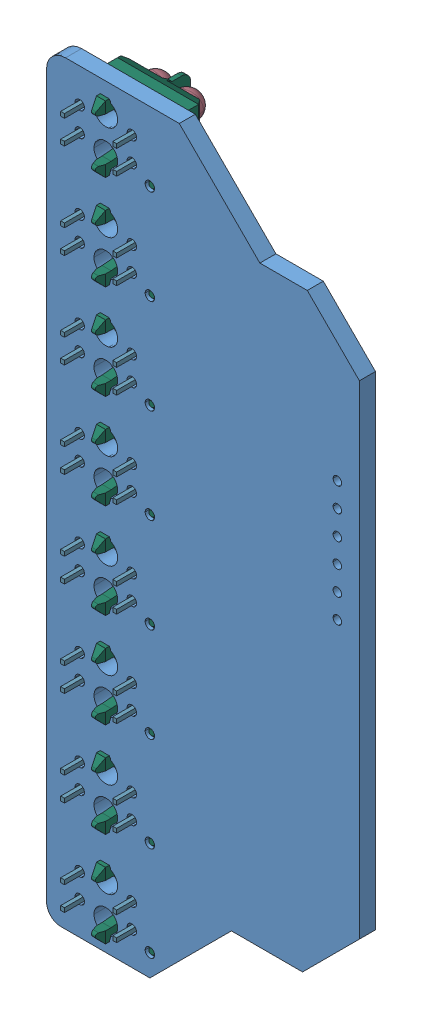
SolidWorks assembly Linelance_PCB v1.1, configuration По умолчанию. Lengths in mm.
Overall size (33 79.6 10.52).
455 component instances, 37 part files, 0 mates.
Components (placement in the parent):
- Linelance_PCB v1.1.step-1: Linelance_PCB v1.1.step [По умолчанию] at origin size (33 79.6 10.52)
  - Linelance_PCB v1.1.step.step-1: Linelance_PCB v1.1.step.step [По умолчанию] at origin size (33 79.6 10.52)
    - Board.step.step-1: Board.step.step [По умолчанию] at origin size (33 79.6 1.69)
      - Open CASCADE STEP translator 6.8 2.1.1.step.step-1: Open CASCADE STEP translator 6.8 2.1.1.step.step [По умолчанию] at (0 0 -1.692) size (33 79.6 1.69)
    - C16.step.step-1: C16.step.step [По умолчанию] at origin size (1.6 0.8 0.5)
      - 5899458880.step.step-1: 5899458880.step.step [По умолчанию] at (18.6 33.5 -2.192) size (1 0.8 0.5)
        - Extruded.step.step-1: Extruded.step.step [По умолчанию] at origin size (1 0.8 0.5)
      - 5899458400.step.step-1: 5899458400.step.step [По умолчанию] at (19.25 33.5 -2.192) size (0.3 0.8 0.5)
        - Extruded-0.step.step-1: Extruded-0.step.step [По умолчанию] at origin size (0.3 0.8 0.5)
      - 5899458400.step-1.step-1: 5899458400.step-1.step [По умолчанию] at (17.95 33.5 -2.192) size (0.3 0.8 0.5)
        - Extruded-0.step.step-1: Extruded-0.step.step [По умолчанию] at origin size (0.3 0.8 0.5)
    - C15.step.step-1: C15.step.step [По умолчанию] at origin size (1.6 0.8 0.5)
      - 5899458880.step-1.step-1: 5899458880.step-1.step [По умолчанию] at (18.6 34.8 -2.192) size (1 0.8 0.5)
        - Extruded.step.step-1: Extruded.step.step [По умолчанию] at origin size (1 0.8 0.5)
      - 5899458400.step-2.step-1: 5899458400.step-2.step [По умолчанию] at (19.25 34.8 -2.192) size (0.3 0.8 0.5)
        - Extruded-0.step.step-1: Extruded-0.step.step [По умолчанию] at origin size (0.3 0.8 0.5)
      - 5899458400.step-3.step-1: 5899458400.step-3.step [По умолчанию] at (17.95 34.8 -2.192) size (0.3 0.8 0.5)
        - Extruded-0.step.step-1: Extruded-0.step.step [По умолчанию] at origin size (0.3 0.8 0.5)
    - C11.step.step-1: C11.step.step [По умолчанию] at origin size (0.8 1.6 0.5)
      - 5899457520.step.step-1: 5899457520.step.step [По умолчанию] at (26.2 43.7 -2.192) size (0.8 1 0.5)
        - Extruded-1.step.step-1: Extruded-1.step.step [По умолчанию] at origin size (0.8 1 0.5)
      - 5899457200.step.step-1: 5899457200.step.step [По умолчанию] at (26.2 43.05 -2.192) size (0.8 0.3 0.5)
        - Extruded-2.step.step-1: Extruded-2.step.step [По умолчанию] at origin size (0.8 0.3 0.5)
      - 5899457200.step-1.step-1: 5899457200.step-1.step [По умолчанию] at (26.2 44.35 -2.192) size (0.8 0.3 0.5)
        - Extruded-2.step.step-1: Extruded-2.step.step [По умолчанию] at origin size (0.8 0.3 0.5)
    - R1.step.step-1: R1.step.step [По умолчанию] at origin size (1.6 0.8 0.5)
      - 5770196880.step.step-1: 5770196880.step.step [По умолчанию] at (26.3 33.7 -1.692) x (-1 0 0) z (0 0 -1) size (1.6 0.8 0.5)
        - Terminal.step.step-1: Terminal.step.step [По умолчанию] at (-0.8 -0.4 0) size (0.3 0.8 0.5)
          - Open_CASCADE_STEP_translator_6.8_7.2.1.step.step-1: Open_CASCADE_STEP_translator_6.8_7.2.1.step.step [По умолчанию] at origin size (0.3 0.8 0.5)
        - Terminal.step-1.step-1: Terminal.step-1.step [По умолчанию] at (0.8 0.4 0) x (-1 0 0) z (0 0 1) size (0.3 0.8 0.5)
          - Open_CASCADE_STEP_translator_6.8_7.2.1.step.step-1: Open_CASCADE_STEP_translator_6.8_7.2.1.step.step [По умолчанию] at origin size (0.3 0.8 0.5)
        - Mid_Body.step.step-1: Mid_Body.step.step [По умолчанию] at (-0.8 -0.4 0) size (1.5 0.8 0.4)
        - Mark.step.step-1: Mark.step.step [По умолчанию] at (-0.5 -0.4 0.45) size (1 0.8 0.05)
    - Y1.step.step-1: Y1.step.step [По умолчанию] at origin size (3.2 2.5 0.6)
      - TSX-3225.step.step-1: TSX-3225.step.step [По умолчанию] at (23.15 31 -1.692) x (1 0 0) z (0 0 -1) size (3.2 2.5 0.6)
    - RN2.step.step-1: RN2.step.step [По умолчанию] at origin size (1.85 3.35 0.7)
      - 5770195440.step.step-1: 5770195440.step.step [По умолчанию] at (13.2 19.25 -1.692) x (1 0 0) z (0 0 -1) size (1.85 3.35 0.7)
        - body.step.step-1: body.step.step [По умолчанию] at (-0.875 -1.675 0) size (1.75 3.35 0.6)
          - Open_CASCADE_STEP_translator_6.8_25.1.1.step.step-1: Open_CASCADE_STEP_translator_6.8_25.1.1.step.step [По умолчанию] at origin size (1.75 3.35 0.6)
        - Mid_Pin.step.step-1: Mid_Pin.step.step [По умолчанию] at (-0.875 -1.2 0) size (0.3 0.38 0.7)
          - Open_CASCADE_STEP_translator_6.8_25.3.1.step.step-1: Open_CASCADE_STEP_translator_6.8_25.3.1.step.step [По умолчанию] at origin size (0.3 0.38 0.7)
        - Mid_Pin.step-1.step-1: Mid_Pin.step-1.step [По умолчанию] at (0.875 1.2 0) x (-1 0 0) z (0 0 1) size (0.3 0.38 0.7)
          - Open_CASCADE_STEP_translator_6.8_25.3.1.step.step-1: Open_CASCADE_STEP_translator_6.8_25.3.1.step.step [По умолчанию] at origin size (0.3 0.38 0.7)
        - Mid_Pin.step-2.step-1: Mid_Pin.step-2.step [По умолчанию] at (-0.875 -0.4 0) size (0.3 0.38 0.7)
          - Open_CASCADE_STEP_translator_6.8_25.3.1.step.step-1: Open_CASCADE_STEP_translator_6.8_25.3.1.step.step [По умолчанию] at origin size (0.3 0.38 0.7)
        - Mid_Pin.step-3.step-1: Mid_Pin.step-3.step [По умолчанию] at (0.875 0.4 0) x (-1 0 0) z (0 0 1) size (0.3 0.38 0.7)
          - Open_CASCADE_STEP_translator_6.8_25.3.1.step.step-1: Open_CASCADE_STEP_translator_6.8_25.3.1.step.step [По умолчанию] at origin size (0.3 0.38 0.7)
        - Mid_Pin.step-4.step-1: Mid_Pin.step-4.step [По умолчанию] at (-0.875 0.4 0) size (0.3 0.38 0.7)
          - Open_CASCADE_STEP_translator_6.8_25.3.1.step.step-1: Open_CASCADE_STEP_translator_6.8_25.3.1.step.step [По умолчанию] at origin size (0.3 0.38 0.7)
        - Mid_Pin.step-5.step-1: Mid_Pin.step-5.step [По умолчанию] at (0.875 -0.4 0) x (-1 0 0) z (0 0 1) size (0.3 0.38 0.7)
          - Open_CASCADE_STEP_translator_6.8_25.3.1.step.step-1: Open_CASCADE_STEP_translator_6.8_25.3.1.step.step [По умолчанию] at origin size (0.3 0.38 0.7)
        - Mid_Pin.step-6.step-1: Mid_Pin.step-6.step [По умолчанию] at (-0.875 1.2 0) size (0.3 0.38 0.7)
          - Open_CASCADE_STEP_translator_6.8_25.3.1.step.step-1: Open_CASCADE_STEP_translator_6.8_25.3.1.step.step [По умолчанию] at origin size (0.3 0.38 0.7)
        - Mid_Pin.step-7.step-1: Mid_Pin.step-7.step [По умолчанию] at (0.875 -1.2 0) x (-1 0 0) z (0 0 1) size (0.3 0.38 0.7)
          - Open_CASCADE_STEP_translator_6.8_25.3.1.step.step-1: Open_CASCADE_STEP_translator_6.8_25.3.1.step.step [По умолчанию] at origin size (0.3 0.38 0.7)
        - Mark.step.step-1: Mark.step.step [По умолчанию] at (-0.875 -1.675 0) size (1 0.8 0.05)
    - RN1.step.step-1: RN1.step.step [По умолчанию] at origin size (1.85 3.35 0.7)
      - 5770195440.step-1.step-1: 5770195440.step-1.step [По умолчанию] at (13.3 61.4 -1.692) x (1 0 0) z (0 0 -1) size (1.85 3.35 0.7)
        - body.step-1.step-1: body.step-1.step [По умолчанию] at (-0.875 -1.675 0) size (1.75 3.35 0.6)
          - Open_CASCADE_STEP_translator_6.8_25.1.1.step.step-1: Open_CASCADE_STEP_translator_6.8_25.1.1.step.step [По умолчанию] at origin size (1.75 3.35 0.6)
        - Mid_Pin.step-8.step-1: Mid_Pin.step-8.step [По умолчанию] at (-0.875 -1.2 0) size (0.3 0.38 0.7)
          - Open_CASCADE_STEP_translator_6.8_25.3.1.step.step-1: Open_CASCADE_STEP_translator_6.8_25.3.1.step.step [По умолчанию] at origin size (0.3 0.38 0.7)
        - Mid_Pin.step-9.step-1: Mid_Pin.step-9.step [По умолчанию] at (0.875 1.2 0) x (-1 0 0) z (0 0 1) size (0.3 0.38 0.7)
          - Open_CASCADE_STEP_translator_6.8_25.3.1.step.step-1: Open_CASCADE_STEP_translator_6.8_25.3.1.step.step [По умолчанию] at origin size (0.3 0.38 0.7)
        - Mid_Pin.step-10.step-1: Mid_Pin.step-10.step [По умолчанию] at (-0.875 -0.4 0) size (0.3 0.38 0.7)
          - Open_CASCADE_STEP_translator_6.8_25.3.1.step.step-1: Open_CASCADE_STEP_translator_6.8_25.3.1.step.step [По умолчанию] at origin size (0.3 0.38 0.7)
        - Mid_Pin.step-11.step-1: Mid_Pin.step-11.step [По умолчанию] at (0.875 0.4 0) x (-1 0 0) z (0 0 1) size (0.3 0.38 0.7)
          - Open_CASCADE_STEP_translator_6.8_25.3.1.step.step-1: Open_CASCADE_STEP_translator_6.8_25.3.1.step.step [По умолчанию] at origin size (0.3 0.38 0.7)
        - Mid_Pin.step-12.step-1: Mid_Pin.step-12.step [По умолчанию] at (-0.875 0.4 0) size (0.3 0.38 0.7)
          - Open_CASCADE_STEP_translator_6.8_25.3.1.step.step-1: Open_CASCADE_STEP_translator_6.8_25.3.1.step.step [По умолчанию] at origin size (0.3 0.38 0.7)
        - Mid_Pin.step-13.step-1: Mid_Pin.step-13.step [По умолчанию] at (0.875 -0.4 0) x (-1 0 0) z (0 0 1) size (0.3 0.38 0.7)
          - Open_CASCADE_STEP_translator_6.8_25.3.1.step.step-1: Open_CASCADE_STEP_translator_6.8_25.3.1.step.step [По умолчанию] at origin size (0.3 0.38 0.7)
        - Mid_Pin.step-14.step-1: Mid_Pin.step-14.step [По умолчанию] at (-0.875 1.2 0) size (0.3 0.38 0.7)
          - Open_CASCADE_STEP_translator_6.8_25.3.1.step.step-1: Open_CASCADE_STEP_translator_6.8_25.3.1.step.step [По умолчанию] at origin size (0.3 0.38 0.7)
        - Mid_Pin.step-15.step-1: Mid_Pin.step-15.step [По умолчанию] at (0.875 -1.2 0) x (-1 0 0) z (0 0 1) size (0.3 0.38 0.7)
          - Open_CASCADE_STEP_translator_6.8_25.3.1.step.step-1: Open_CASCADE_STEP_translator_6.8_25.3.1.step.step [По умолчанию] at origin size (0.3 0.38 0.7)
        - Mark.step.step-1: Mark.step.step [По умолчанию] at (-0.875 -1.675 0) size (1 0.8 0.05)
    - C23.step.step-1: C23.step.step [По умолчанию] at origin size (1.6 0.8 0.5)
      - 5899458400.step-4.step-1: 5899458400.step-4.step [По умолчанию] at (17.5 13.375 -2.192) size (0.3 0.8 0.5)
        - Extruded-0.step.step-1: Extruded-0.step.step [По умолчанию] at origin size (0.3 0.8 0.5)
      - 5899458400.step-5.step-1: 5899458400.step-5.step [По умолчанию] at (16.2 13.375 -2.192) size (0.3 0.8 0.5)
        - Extruded-0.step.step-1: Extruded-0.step.step [По умолчанию] at origin size (0.3 0.8 0.5)
      - 5899458880.step-2.step-1: 5899458880.step-2.step [По умолчанию] at (16.85 13.375 -2.192) size (1 0.8 0.5)
        - Extruded.step.step-1: Extruded.step.step [По умолчанию] at origin size (1 0.8 0.5)
    - C22.step.step-1: C22.step.step [По умолчанию] at origin size (1.6 0.8 0.5)
      - 5899458400.step-6.step-1: 5899458400.step-6.step [По умолчанию] at (17.625 57.7 -2.192) size (0.3 0.8 0.5)
        - Extruded-0.step.step-1: Extruded-0.step.step [По умолчанию] at origin size (0.3 0.8 0.5)
      - 5899458400.step-7.step-1: 5899458400.step-7.step [По умолчанию] at (16.325 57.7 -2.192) size (0.3 0.8 0.5)
        - Extruded-0.step.step-1: Extruded-0.step.step [По умолчанию] at origin size (0.3 0.8 0.5)
      - 5899458880.step-3.step-1: 5899458880.step-3.step [По умолчанию] at (16.975 57.7 -2.192) size (1 0.8 0.5)
        - Extruded.step.step-1: Extruded.step.step [По умолчанию] at origin size (1 0.8 0.5)
    - Q9.step.step-1: Q9.step.step [По умолчанию] at origin size (2.3 2.9 1)
      - SOT23-3.step.step-1: SOT23-3.step.step [По умолчанию] at (13.2 10.85 -1.692) x (0 -1 0) z (1 0 0) size (2.9 1 2.3)
    - Q8.step.step-1: Q8.step.step [По умолчанию] at origin size (2.9 2.3 1)
      - SOT23-3.step.step-1: SOT23-3.step.step [По умолчанию] at (14.75 14.925 -1.692) x (-1 0 0) z (0 -1 0) size (2.9 1 2.3)
    - Q7.step.step-1: Q7.step.step [По умолчанию] at origin size (2.9 2.3 1)
      - SOT23-3.step.step-1: SOT23-3.step.step [По умолчанию] at (15 25.2 -1.692) x (-1 0 0) z (0 -1 0) size (2.9 1 2.3)
    - Q6.step.step-1: Q6.step.step [По умолчанию] at origin size (2.9 2.3 1)
      - SOT23-3.step.step-1: SOT23-3.step.step [По умолчанию] at (15 35.2 -1.692) x (-1 0 0) z (0 -1 0) size (2.9 1 2.3)
    - Q4.step.step-1: Q4.step.step [По умолчанию] at origin size (2.9 2.3 1)
      - SOT23-3.step.step-1: SOT23-3.step.step [По умолчанию] at (15.05 55 -1.692) x (-1 0 0) z (0 -1 0) size (2.9 1 2.3)
    - Q5.step.step-1: Q5.step.step [По умолчанию] at origin size (2.9 2.3 1)
      - SOT23-3.step.step-1: SOT23-3.step.step [По умолчанию] at (15.05 40.9 -1.692) x (-1 0 0) z (0 -1 0) size (2.9 1 2.3)
    - Q3.step.step-1: Q3.step.step [По умолчанию] at origin size (2.3 2.9 1)
      - SOT23-3.step.step-1: SOT23-3.step.step [По умолчанию] at (13.8 69.6 -1.692) x (0 -1 0) z (1 0 0) size (2.9 1 2.3)
    - Q2.step.step-1: Q2.step.step [По умолчанию] at origin size (2.9 2.3 1)
      - SOT23-3.step.step-1: SOT23-3.step.step [По умолчанию] at (15 75.2 -1.692) x (-1 0 0) z (0 -1 0) size (2.9 1 2.3)
    - U12.step.step-1: U12.step.step [По умолчанию] at origin size (10.2 7 10.52)
      - TCRT5000.step.step-1: TCRT5000.step.step [По умолчанию] at (6.25 4.77 -1.692) x (0 1 0) z (-1 0 0) size (7 10.52 10.2)
        - LEDs.step.step-1: LEDs.step.step [По умолчанию] at origin size (2.8 2.98 6.71)
        - Metal_Contacts.step.step-1: Metal_Contacts.step.step [По умолчанию] at origin size (3.19 4.01 5.9)
        - Open CASCADE STEP translator 6.8 2.19.1.3.step.step-1: Open CASCADE STEP translator 6.8 2.19.1.3.step.step [По умолчанию] at origin size (7 10.13 10.2)
    - U11.step.step-1: U11.step.step [По умолчанию] at origin size (10.2 7 10.52)
      - TCRT5000.step-1.step-1: TCRT5000.step-1.step [По умолчанию] at (6.25 14.77 -1.692) x (0 1 0) z (-1 0 0) size (7 10.52 10.2)
        - LEDs.step.step-1: LEDs.step.step [По умолчанию] at origin size (2.8 2.98 6.71)
        - Metal_Contacts.step.step-1: Metal_Contacts.step.step [По умолчанию] at origin size (3.19 4.01 5.9)
        - Open CASCADE STEP translator 6.8 2.19.1.3.step.step-1: Open CASCADE STEP translator 6.8 2.19.1.3.step.step [По умолчанию] at origin size (7 10.13 10.2)
    - U10.step.step-1: U10.step.step [По умолчанию] at origin size (10.2 7 10.52)
      - TCRT5000.step-2.step-1: TCRT5000.step-2.step [По умолчанию] at (6.25 24.77 -1.692) x (0 1 0) z (-1 0 0) size (7 10.52 10.2)
        - LEDs.step.step-1: LEDs.step.step [По умолчанию] at origin size (2.8 2.98 6.71)
        - Metal_Contacts.step.step-1: Metal_Contacts.step.step [По умолчанию] at origin size (3.19 4.01 5.9)
        - Open CASCADE STEP translator 6.8 2.19.1.3.step.step-1: Open CASCADE STEP translator 6.8 2.19.1.3.step.step [По умолчанию] at origin size (7 10.13 10.2)
    - U9.step.step-1: U9.step.step [По умолчанию] at origin size (10.2 7 10.52)
      - TCRT5000.step-3.step-1: TCRT5000.step-3.step [По умолчанию] at (6.25 34.77 -1.692) x (0 1 0) z (-1 0 0) size (7 10.52 10.2)
        - LEDs.step.step-1: LEDs.step.step [По умолчанию] at origin size (2.8 2.98 6.71)
        - Metal_Contacts.step.step-1: Metal_Contacts.step.step [По умолчанию] at origin size (3.19 4.01 5.9)
        - Open CASCADE STEP translator 6.8 2.19.1.3.step.step-1: Open CASCADE STEP translator 6.8 2.19.1.3.step.step [По умолчанию] at origin size (7 10.13 10.2)
    - U7.step.step-1: U7.step.step [По умолчанию] at origin size (10.2 7 10.52)
      - TCRT5000.step-4.step-1: TCRT5000.step-4.step [По умолчанию] at (6.25 54.77 -1.692) x (0 1 0) z (-1 0 0) size (7 10.52 10.2)
        - LEDs.step.step-1: LEDs.step.step [По умолчанию] at origin size (2.8 2.98 6.71)
        - Metal_Contacts.step.step-1: Metal_Contacts.step.step [По умолчанию] at origin size (3.19 4.01 5.9)
        - Open CASCADE STEP translator 6.8 2.19.1.3.step.step-1: Open CASCADE STEP translator 6.8 2.19.1.3.step.step [По умолчанию] at origin size (7 10.13 10.2)
    - U8.step.step-1: U8.step.step [По умолчанию] at origin size (10.2 7 10.52)
      - TCRT5000.step-5.step-1: TCRT5000.step-5.step [По умолчанию] at (6.25 44.77 -1.692) x (0 1 0) z (-1 0 0) size (7 10.52 10.2)
        - LEDs.step.step-1: LEDs.step.step [По умолчанию] at origin size (2.8 2.98 6.71)
        - Metal_Contacts.step.step-1: Metal_Contacts.step.step [По умолчанию] at origin size (3.19 4.01 5.9)
        - Open CASCADE STEP translator 6.8 2.19.1.3.step.step-1: Open CASCADE STEP translator 6.8 2.19.1.3.step.step [По умолчанию] at origin size (7 10.13 10.2)
    - U6.step.step-1: U6.step.step [По умолчанию] at origin size (10.2 7 10.52)
      - TCRT5000.step-6.step-1: TCRT5000.step-6.step [По умолчанию] at (6.25 64.77 -1.692) x (0 1 0) z (-1 0 0) size (7 10.52 10.2)
        - LEDs.step.step-1: LEDs.step.step [По умолчанию] at origin size (2.8 2.98 6.71)
        - Metal_Contacts.step.step-1: Metal_Contacts.step.step [По умолчанию] at origin size (3.19 4.01 5.9)
        - Open CASCADE STEP translator 6.8 2.19.1.3.step.step-1: Open CASCADE STEP translator 6.8 2.19.1.3.step.step [По умолчанию] at origin size (7 10.13 10.2)
    - U5.step.step-1: U5.step.step [По умолчанию] at origin size (10.2 7 10.52)
      - TCRT5000.step-7.step-1: TCRT5000.step-7.step [По умолчанию] at (6.25 74.77 -1.692) x (0 1 0) z (-1 0 0) size (7 10.52 10.2)
        - LEDs.step.step-1: LEDs.step.step [По умолчанию] at origin size (2.8 2.98 6.71)
        - Metal_Contacts.step.step-1: Metal_Contacts.step.step [По умолчанию] at origin size (3.19 4.01 5.9)
        - Open CASCADE STEP translator 6.8 2.19.1.3.step.step-1: Open CASCADE STEP translator 6.8 2.19.1.3.step.step [По умолчанию] at origin size (7 10.13 10.2)
    - Q1.step.step-1: Q1.step.step [По умолчанию] at origin size (2.9 2.3 1)
      - SOT23-3.step.step-1: SOT23-3.step.step [По умолчанию] at (19.1975 48.8275 -1.692) x (1 0 0) z (0 1 0) size (2.9 1 2.3)
    - U2.step.step-1: U2.step.step [По умолчанию] at origin size (2.5 3 1.1)
      - SOT23-5.step.step-1: SOT23-5.step.step [По умолчанию] at (17.7001 44.6999 -2.232) x (0 1 0) z (-1 0 0) size (3 1.1 2.5)
    - DA1.step.step-1: DA1.step.step [По умолчанию] at origin size (3 2.5 1.1)
      - SOT23-5.step.step-1: SOT23-5.step.step [По умолчанию] at (26.651 51.0529 -2.232) x (1 0 0) z (0 1 0) size (3 1.1 2.5)
    - C1.step.step-1: C1.step.step [По умолчанию] at origin size (1.8 4.8 1.84)
      - TANT-A.step.step-1: TANT-A.step.step [По умолчанию] at (27.6 56.9073 -1.692) x (0 -1 0) z (0 0 -1) size (4.8 1.8 1.84)
    - C4.step.step-1: C4.step.step [По умолчанию] at origin size (1.8 4.8 1.84)
      - TANT-A.step.step-1: TANT-A.step.step [По умолчанию] at (23.6 49.45 -1.692) x (0 1 0) z (0 0 -1) size (4.8 1.8 1.84)
    - U4.step.step-1: U4.step.step [По умолчанию] at origin size (8.49 6 1.66)
      - 5770194960.step.step-1: 5770194960.step.step [По умолчанию] at (19.8415 17.835 -1.692) x (0 -1 0) z (0 0 -1) size (6 8.48 1.66)
        - body.step-2.step-1: body.step-2.step [По умолчанию] at (-2 -4.4 0) size (1.75 3.35 0.6)
          - Open_CASCADE_STEP_translator_6.8_25.1.1.step.step-1: Open_CASCADE_STEP_translator_6.8_25.1.1.step.step [По умолчанию] at origin size (1.75 3.35 0.6)
        - Open_CASCADE_STEP_translator_6.8_12.1.step.step-1: Open_CASCADE_STEP_translator_6.8_12.1.step.step [По умолчанию] at (-2 -4.4 0.001) size (0.51 0.51 0.01)
        - Leader.step.step-1: Leader.step.step [По умолчанию] at (-2 -3.81 0) x (-1 0 0) z (0 0 1) size (1 0.55 0.97)
        - Leader.step.step-2: Leader.step.step [По умолчанию] at (-2 -2.54 0) x (-1 0 0) z (0 0 1) size (1 0.55 0.97)
        - Leader.step.step-3: Leader.step.step [По умолчанию] at (-2 -1.27 0) x (-1 0 0) z (0 0 1) size (1 0.55 0.97)
        - Leader.step.step-4: Leader.step.step [По умолчанию] at (-2 0 0) x (-1 0 0) z (0 0 1) size (1 0.55 0.97)
        - Leader.step.step-5: Leader.step.step [По умолчанию] at (-2 1.27 0) x (-1 0 0) z (0 0 1) size (1 0.55 0.97)
        - Leader.step.step-6: Leader.step.step [По умолчанию] at (-2 2.54 0) x (-1 0 0) z (0 0 1) size (1 0.55 0.97)
        - Leader.step.step-7: Leader.step.step [По умолчанию] at (-2 3.81 0) x (-1 0 0) z (0 0 1) size (1 0.55 0.97)
        - Leader.step.step-8: Leader.step.step [По умолчанию] at (2 -3.81 0) size (1 0.55 0.97)
        - Leader.step.step-9: Leader.step.step [По умолчанию] at (2 -2.54 0) size (1 0.55 0.97)
        - Leader.step.step-10: Leader.step.step [По умолчанию] at (2 -1.27 0) size (1 0.55 0.97)
        - Leader.step.step-11: Leader.step.step [По умолчанию] at (2 0 0) size (1 0.55 0.97)
        - Leader.step.step-12: Leader.step.step [По умолчанию] at (2 1.27 0) size (1 0.55 0.97)
        - Leader.step.step-13: Leader.step.step [По умолчанию] at (2 2.54 0) size (1 0.55 0.97)
        - Leader.step.step-14: Leader.step.step [По умолчанию] at (2 3.81 0) size (1 0.55 0.97)
    - U3.step.step-1: U3.step.step [По умолчанию] at origin size (8.49 6 1.66)
      - 5770194960.step-1.step-1: 5770194960.step-1.step [По умолчанию] at (19.9415 62.135 -1.692) x (0 -1 0) z (0 0 -1) size (6 8.48 1.66)
        - body.step-3.step-1: body.step-3.step [По умолчанию] at (-2 -4.4 0) size (1.75 3.35 0.6)
          - Open_CASCADE_STEP_translator_6.8_25.1.1.step.step-1: Open_CASCADE_STEP_translator_6.8_25.1.1.step.step [По умолчанию] at origin size (1.75 3.35 0.6)
        - Open_CASCADE_STEP_translator_6.8_12.1.step.step-1: Open_CASCADE_STEP_translator_6.8_12.1.step.step [По умолчанию] at (-2 -4.4 0.001) size (0.51 0.51 0.01)
        - Leader.step.step-1: Leader.step.step [По умолчанию] at (-2 -3.81 0) x (-1 0 0) z (0 0 1) size (1 0.55 0.97)
        - Leader.step.step-2: Leader.step.step [По умолчанию] at (-2 -2.54 0) x (-1 0 0) z (0 0 1) size (1 0.55 0.97)
        - Leader.step.step-3: Leader.step.step [По умолчанию] at (-2 -1.27 0) x (-1 0 0) z (0 0 1) size (1 0.55 0.97)
        - Leader.step.step-4: Leader.step.step [По умолчанию] at (-2 0 0) x (-1 0 0) z (0 0 1) size (1 0.55 0.97)
        - Leader.step.step-5: Leader.step.step [По умолчанию] at (-2 1.27 0) x (-1 0 0) z (0 0 1) size (1 0.55 0.97)
        - Leader.step.step-6: Leader.step.step [По умолчанию] at (-2 2.54 0) x (-1 0 0) z (0 0 1) size (1 0.55 0.97)
        - Leader.step.step-7: Leader.step.step [По умолчанию] at (-2 3.81 0) x (-1 0 0) z (0 0 1) size (1 0.55 0.97)
        - Leader.step.step-8: Leader.step.step [По умолчанию] at (2 -3.81 0) size (1 0.55 0.97)
        - Leader.step.step-9: Leader.step.step [По умолчанию] at (2 -2.54 0) size (1 0.55 0.97)
        - Leader.step.step-10: Leader.step.step [По умолчанию] at (2 -1.27 0) size (1 0.55 0.97)
        - Leader.step.step-11: Leader.step.step [По умолчанию] at (2 0 0) size (1 0.55 0.97)
        - Leader.step.step-12: Leader.step.step [По умолчанию] at (2 1.27 0) size (1 0.55 0.97)
        - Leader.step.step-13: Leader.step.step [По умолчанию] at (2 2.54 0) size (1 0.55 0.97)
        - Leader.step.step-14: Leader.step.step [По умолчанию] at (2 3.81 0) size (1 0.55 0.97)
    - U1.step.step-1: U1.step.step [По умолчанию] at origin size (6.4 6.5 1.1)
      - TSSOP-20.step.step-1: TSSOP-20.step.step [По умолчанию] at (24.9249 35.125 -1.692) x (0 1 0) z (-1 0 0) size (6.5 1.1 6.4)
    - RESET.step.step-1: RESET.step.step [По умолчанию] at origin size (4.6 2.8 1.94)
      - KMR221GLFS.step.step-1: KMR221GLFS.step.step [По умолчанию] at (23.6249 25.1001 -1.692) x (-1 0 0) z (0 -1 0) size (4.6 1.94 2.8)
    - BOOT0.step.step-1: BOOT0.step.step [По умолчанию] at origin size (4.6 2.8 1.94)
      - KMR221GLFS.step.step-1: KMR221GLFS.step.step [По умолчанию] at (29.3999 25.1001 -1.692) x (-1 0 0) z (0 -1 0) size (4.6 1.94 2.8)
    - R15.step.step-1: R15.step.step [По умолчанию] at origin size (0.8 1.6 0.5)
      - 5770195520.step.step-1: 5770195520.step.step [По умолчанию] at (3.4 9.8 -1.692) x (0 1 0) z (0 0 -1) size (1.6 0.8 0.5)
        - Terminal-1.step.step-1: Terminal-1.step.step [По умолчанию] at (-0.8 -0.4 0) size (0.3 0.8 0.5)
          - Open_CASCADE_STEP_translator_6.8_7.2.1-3.step.step-1: Open_CASCADE_STEP_translator_6.8_7.2.1-3.step.step [По умолчанию] at origin size (0.3 0.8 0.5)
        - Terminal-1.step-1.step-1: Terminal-1.step-1.step [По умолчанию] at (0.8 0.4 0) x (-1 0 0) z (0 0 1) size (0.3 0.8 0.5)
          - Open_CASCADE_STEP_translator_6.8_7.2.1-3.step.step-1: Open_CASCADE_STEP_translator_6.8_7.2.1-3.step.step [По умолчанию] at origin size (0.3 0.8 0.5)
        - Mid_Body-4.step.step-1: Mid_Body-4.step.step [По умолчанию] at (-0.8 -0.4 0) size (1.5 0.8 0.4)
        - Mark-5.step.step-1: Mark-5.step.step [По умолчанию] at (-0.5 -0.4 0.45) size (1 0.8 0.05)
    - R14.step.step-1: R14.step.step [По умолчанию] at origin size (0.8 1.6 0.5)
      - 5770190160.step.step-1: 5770190160.step.step [По умолчанию] at (4.8 9.8 -1.692) x (0 -1 0) z (0 0 -1) size (1.6 0.8 0.5)
        - Terminal-2.step.step-1: Terminal-2.step.step [По умолчанию] at (-0.8 -0.4 0) size (0.3 0.8 0.5)
          - Open_CASCADE_STEP_translator_6.8_7.2.1-6.step.step-1: Open_CASCADE_STEP_translator_6.8_7.2.1-6.step.step [По умолчанию] at origin size (0.3 0.8 0.5)
        - Terminal-2.step-1.step-1: Terminal-2.step-1.step [По умолчанию] at (0.8 0.4 0) x (-1 0 0) z (0 0 1) size (0.3 0.8 0.5)
          - Open_CASCADE_STEP_translator_6.8_7.2.1-6.step.step-1: Open_CASCADE_STEP_translator_6.8_7.2.1-6.step.step [По умолчанию] at origin size (0.3 0.8 0.5)
        - Mid_Body-7.step.step-1: Mid_Body-7.step.step [По умолчанию] at (-0.8 -0.4 0) size (1.5 0.8 0.4)
        - Mark-8.step.step-1: Mark-8.step.step [По умолчанию] at (-0.5 -0.4 0.45) size (1 0.8 0.05)
    - R13.step.step-1: R13.step.step [По умолчанию] at origin size (0.8 1.6 0.5)
      - 5770190160.step-1.step-1: 5770190160.step-1.step [По умолчанию] at (4.2 19.8 -1.692) x (0 -1 0) z (0 0 -1) size (1.6 0.8 0.5)
        - Terminal-2.step-2.step-1: Terminal-2.step-2.step [По умолчанию] at (-0.8 -0.4 0) size (0.3 0.8 0.5)
          - Open_CASCADE_STEP_translator_6.8_7.2.1-6.step.step-1: Open_CASCADE_STEP_translator_6.8_7.2.1-6.step.step [По умолчанию] at origin size (0.3 0.8 0.5)
        - Terminal-2.step-3.step-1: Terminal-2.step-3.step [По умолчанию] at (0.8 0.4 0) x (-1 0 0) z (0 0 1) size (0.3 0.8 0.5)
          - Open_CASCADE_STEP_translator_6.8_7.2.1-6.step.step-1: Open_CASCADE_STEP_translator_6.8_7.2.1-6.step.step [По умолчанию] at origin size (0.3 0.8 0.5)
        - Mid_Body-7.step.step-1: Mid_Body-7.step.step [По умолчанию] at (-0.8 -0.4 0) size (1.5 0.8 0.4)
        - Mark-8.step.step-1: Mark-8.step.step [По умолчанию] at (-0.5 -0.4 0.45) size (1 0.8 0.05)
    - R11.step.step-1: R11.step.step [По умолчанию] at origin size (0.8 1.6 0.5)
      - 5770190160.step-2.step-1: 5770190160.step-2.step [По умолчанию] at (4.2 39.8 -1.692) x (0 -1 0) z (0 0 -1) size (1.6 0.8 0.5)
        - Terminal-2.step-4.step-1: Terminal-2.step-4.step [По умолчанию] at (-0.8 -0.4 0) size (0.3 0.8 0.5)
          - Open_CASCADE_STEP_translator_6.8_7.2.1-6.step.step-1: Open_CASCADE_STEP_translator_6.8_7.2.1-6.step.step [По умолчанию] at origin size (0.3 0.8 0.5)
        - Terminal-2.step-5.step-1: Terminal-2.step-5.step [По умолчанию] at (0.8 0.4 0) x (-1 0 0) z (0 0 1) size (0.3 0.8 0.5)
          - Open_CASCADE_STEP_translator_6.8_7.2.1-6.step.step-1: Open_CASCADE_STEP_translator_6.8_7.2.1-6.step.step [По умолчанию] at origin size (0.3 0.8 0.5)
        - Mid_Body-7.step.step-1: Mid_Body-7.step.step [По умолчанию] at (-0.8 -0.4 0) size (1.5 0.8 0.4)
        - Mark-8.step.step-1: Mark-8.step.step [По умолчанию] at (-0.5 -0.4 0.45) size (1 0.8 0.05)
    - R12.step.step-1: R12.step.step [По умолчанию] at origin size (0.8 1.6 0.5)
      - 5770190160.step-3.step-1: 5770190160.step-3.step [По умолчанию] at (4.2 29.8 -1.692) x (0 -1 0) z (0 0 -1) size (1.6 0.8 0.5)
        - Terminal-2.step-6.step-1: Terminal-2.step-6.step [По умолчанию] at (-0.8 -0.4 0) size (0.3 0.8 0.5)
          - Open_CASCADE_STEP_translator_6.8_7.2.1-6.step.step-1: Open_CASCADE_STEP_translator_6.8_7.2.1-6.step.step [По умолчанию] at origin size (0.3 0.8 0.5)
        - Terminal-2.step-7.step-1: Terminal-2.step-7.step [По умолчанию] at (0.8 0.4 0) x (-1 0 0) z (0 0 1) size (0.3 0.8 0.5)
          - Open_CASCADE_STEP_translator_6.8_7.2.1-6.step.step-1: Open_CASCADE_STEP_translator_6.8_7.2.1-6.step.step [По умолчанию] at origin size (0.3 0.8 0.5)
        - Mid_Body-7.step.step-1: Mid_Body-7.step.step [По умолчанию] at (-0.8 -0.4 0) size (1.5 0.8 0.4)
        - Mark-8.step.step-1: Mark-8.step.step [По умолчанию] at (-0.5 -0.4 0.45) size (1 0.8 0.05)
    - R9.step.step-1: R9.step.step [По умолчанию] at origin size (0.8 1.6 0.5)
      - 5770190160.step-4.step-1: 5770190160.step-4.step [По умолчанию] at (4.2 59.8 -1.692) x (0 -1 0) z (0 0 -1) size (1.6 0.8 0.5)
        - Terminal-2.step-8.step-1: Terminal-2.step-8.step [По умолчанию] at (-0.8 -0.4 0) size (0.3 0.8 0.5)
          - Open_CASCADE_STEP_translator_6.8_7.2.1-6.step.step-1: Open_CASCADE_STEP_translator_6.8_7.2.1-6.step.step [По умолчанию] at origin size (0.3 0.8 0.5)
        - Terminal-2.step-9.step-1: Terminal-2.step-9.step [По умолчанию] at (0.8 0.4 0) x (-1 0 0) z (0 0 1) size (0.3 0.8 0.5)
          - Open_CASCADE_STEP_translator_6.8_7.2.1-6.step.step-1: Open_CASCADE_STEP_translator_6.8_7.2.1-6.step.step [По умолчанию] at origin size (0.3 0.8 0.5)
        - Mid_Body-7.step.step-1: Mid_Body-7.step.step [По умолчанию] at (-0.8 -0.4 0) size (1.5 0.8 0.4)
        - Mark-8.step.step-1: Mark-8.step.step [По умолчанию] at (-0.5 -0.4 0.45) size (1 0.8 0.05)
    - R10.step.step-1: R10.step.step [По умолчанию] at origin size (0.8 1.6 0.5)
      - 5770190160.step-5.step-1: 5770190160.step-5.step [По умолчанию] at (4.2 49.8 -1.692) x (0 -1 0) z (0 0 -1) size (1.6 0.8 0.5)
        - Terminal-2.step-10.step-1: Terminal-2.step-10.step [По умолчанию] at (-0.8 -0.4 0) size (0.3 0.8 0.5)
          - Open_CASCADE_STEP_translator_6.8_7.2.1-6.step.step-1: Open_CASCADE_STEP_translator_6.8_7.2.1-6.step.step [По умолчанию] at origin size (0.3 0.8 0.5)
        - Terminal-2.step-11.step-1: Terminal-2.step-11.step [По умолчанию] at (0.8 0.4 0) x (-1 0 0) z (0 0 1) size (0.3 0.8 0.5)
          - Open_CASCADE_STEP_translator_6.8_7.2.1-6.step.step-1: Open_CASCADE_STEP_translator_6.8_7.2.1-6.step.step [По умолчанию] at origin size (0.3 0.8 0.5)
        - Mid_Body-7.step.step-1: Mid_Body-7.step.step [По умолчанию] at (-0.8 -0.4 0) size (1.5 0.8 0.4)
        - Mark-8.step.step-1: Mark-8.step.step [По умолчанию] at (-0.5 -0.4 0.45) size (1 0.8 0.05)
    - R8.step.step-1: R8.step.step [По умолчанию] at origin size (0.8 1.6 0.5)
